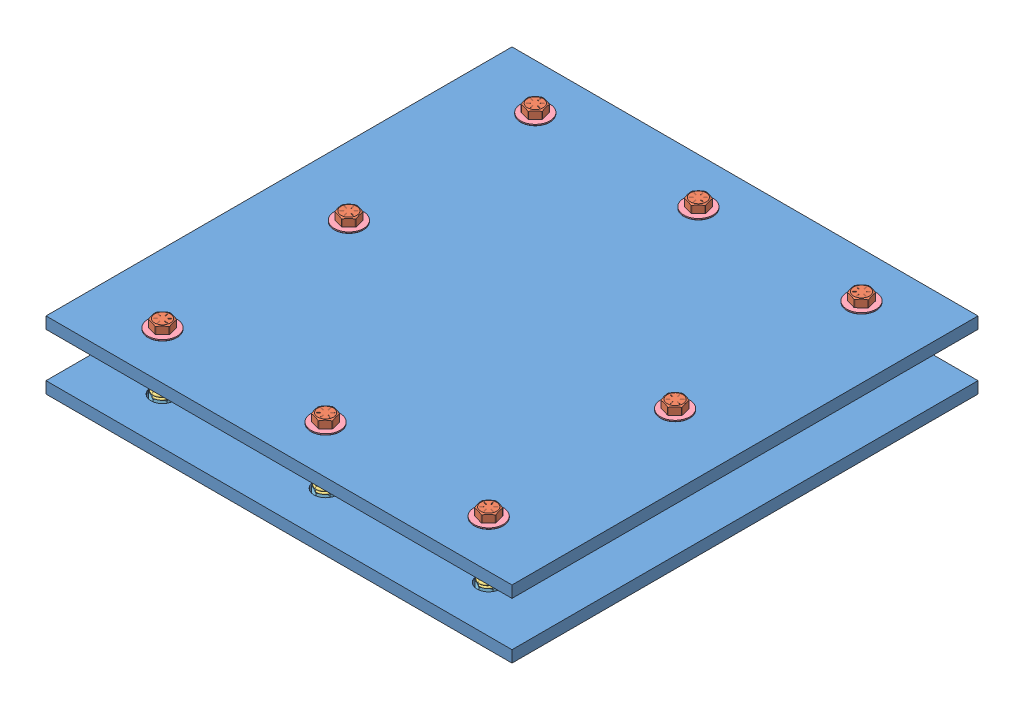
SolidWorks assembly suspension_assem, configuration Default. Lengths in mm.
Overall size (508 85.98 508).
34 component instances, 5 part files, 8 mates.
Components (placement in the parent):
- baseplate-1: baseplate [Default] at (-30.1985 2.5147 9.9128) size (508 12.7 508)
- 92620A724_Zinc Yellow-Chromate Plated Hex Head Screw-1: 92620A724_Zinc Yellow-Chromate Plated Hex Head Screw [92620A724] at (147.6015 16.7895 213.1128) x (0 -1 0) z (-0.270952 0 0.962593) size (85.98 21.7 19.05)
- 9657K31_Compression Spring-1: 9657K31_Compression Spring [9657K31] at (147.6015 12.5847 213.1128) x (-0.104962 0 0.994476) z (0 1 0) size (23.85 23.85 58.72)
- 90107A033_316 Stainless Steel Washer-1: 90107A033_316 Stainless Steel Washer [90107A033] at (147.6015 16.0021 213.1128) x (0.999961 0 0.008869) z (0 -1 0) size (31.75 31.75 1.57)
- 98797A523_Medium-Strength Steel Hex Nuts - Grade 5-1: 98797A523_Medium-Strength Steel Hex Nuts - Grade 5 [98797A523] at (147.6015 -49.9015 213.1128) x (-0.999115 0 0.042064) z (0 -1 0) size (19.05 22 12.65)
- baseplate-2: baseplate [Default] at (-30.1985 -58.6077 9.9128) size (508 12.7 508)
- 98797A523_Medium-Strength Steel Hex Nuts - Grade 5-2: 98797A523_Medium-Strength Steel Hex Nuts - Grade 5 [98797A523] at (147.6015 -49.9015 9.9128) x (-0.999115 0 0.042064) z (0 -1 0) size (19.05 22 12.65)
- 98797A523_Medium-Strength Steel Hex Nuts - Grade 5-3: 98797A523_Medium-Strength Steel Hex Nuts - Grade 5 [98797A523] at (147.6015 -49.9015 -193.2872) x (-0.999115 0 0.042064) z (0 -1 0) size (19.05 22 12.65)
- 98797A523_Medium-Strength Steel Hex Nuts - Grade 5-4: 98797A523_Medium-Strength Steel Hex Nuts - Grade 5 [98797A523] at (-30.1985 -49.9015 213.1128) x (-0.999115 0 0.042064) z (0 -1 0) size (19.05 22 12.65)
- 98797A523_Medium-Strength Steel Hex Nuts - Grade 5-6: 98797A523_Medium-Strength Steel Hex Nuts - Grade 5 [98797A523] at (-30.1985 -49.9015 -193.2872) x (-0.999115 0 0.042064) z (0 -1 0) size (19.05 22 12.65)
- 98797A523_Medium-Strength Steel Hex Nuts - Grade 5-7: 98797A523_Medium-Strength Steel Hex Nuts - Grade 5 [98797A523] at (-207.9985 -49.9015 213.1128) x (-0.999115 0 0.042064) z (0 -1 0) size (19.05 22 12.65)
- 98797A523_Medium-Strength Steel Hex Nuts - Grade 5-8: 98797A523_Medium-Strength Steel Hex Nuts - Grade 5 [98797A523] at (-207.9985 -49.9015 9.9128) x (-0.999115 0 0.042064) z (0 -1 0) size (19.05 22 12.65)
- 98797A523_Medium-Strength Steel Hex Nuts - Grade 5-9: 98797A523_Medium-Strength Steel Hex Nuts - Grade 5 [98797A523] at (-207.9985 -49.9015 -193.2872) x (-0.999115 0 0.042064) z (0 -1 0) size (19.05 22 12.65)
- 9657K31_Compression Spring-2: 9657K31_Compression Spring [9657K31] at (147.6015 12.5847 9.9128) x (-0.104962 0 0.994476) z (0 1 0) size (23.85 23.85 58.72)
- 9657K31_Compression Spring-3: 9657K31_Compression Spring [9657K31] at (147.6015 12.5847 -193.2872) x (-0.104962 0 0.994476) z (0 1 0) size (23.85 23.85 58.72)
- 9657K31_Compression Spring-4: 9657K31_Compression Spring [9657K31] at (-30.1985 12.5847 213.1128) x (-0.104962 0 0.994476) z (0 1 0) size (23.85 23.85 58.72)
- 9657K31_Compression Spring-6: 9657K31_Compression Spring [9657K31] at (-30.1985 12.5847 -193.2872) x (-0.104962 0 0.994476) z (0 1 0) size (23.85 23.85 58.72)
- 9657K31_Compression Spring-7: 9657K31_Compression Spring [9657K31] at (-207.9985 12.5847 213.1128) x (-0.104962 0 0.994476) z (0 1 0) size (23.85 23.85 58.72)
- 9657K31_Compression Spring-8: 9657K31_Compression Spring [9657K31] at (-207.9985 12.5847 9.9128) x (-0.104962 0 0.994476) z (0 1 0) size (23.85 23.85 58.72)
- 9657K31_Compression Spring-9: 9657K31_Compression Spring [9657K31] at (-207.9985 12.5847 -193.2872) x (-0.104962 0 0.994476) z (0 1 0) size (23.85 23.85 58.72)
- 90107A033_316 Stainless Steel Washer-4: 90107A033_316 Stainless Steel Washer [90107A033] at (147.6015 16.0021 9.9128) x (0.999961 0 0.008869) z (0 -1 0) size (31.75 31.75 1.57)
- 90107A033_316 Stainless Steel Washer-5: 90107A033_316 Stainless Steel Washer [90107A033] at (147.6015 16.0021 -193.2872) x (0.999961 0 0.008869) z (0 -1 0) size (31.75 31.75 1.57)
- 90107A033_316 Stainless Steel Washer-6: 90107A033_316 Stainless Steel Washer [90107A033] at (-30.1985 16.0021 213.1128) x (0.999961 0 0.008869) z (0 -1 0) size (31.75 31.75 1.57)
- 90107A033_316 Stainless Steel Washer-8: 90107A033_316 Stainless Steel Washer [90107A033] at (-30.1985 16.0021 -193.2872) x (0.999961 0 0.008869) z (0 -1 0) size (31.75 31.75 1.57)
- 90107A033_316 Stainless Steel Washer-9: 90107A033_316 Stainless Steel Washer [90107A033] at (-207.9985 16.0021 213.1128) x (0.999961 0 0.008869) z (0 -1 0) size (31.75 31.75 1.57)
- 90107A033_316 Stainless Steel Washer-10: 90107A033_316 Stainless Steel Washer [90107A033] at (-207.9985 16.0021 9.9128) x (0.999961 0 0.008869) z (0 -1 0) size (31.75 31.75 1.57)
- 90107A033_316 Stainless Steel Washer-11: 90107A033_316 Stainless Steel Washer [90107A033] at (-207.9985 16.0021 -193.2872) x (0.999961 0 0.008869) z (0 -1 0) size (31.75 31.75 1.57)
- 92620A724_Zinc Yellow-Chromate Plated Hex Head Screw-2: 92620A724_Zinc Yellow-Chromate Plated Hex Head Screw [92620A724] at (147.6015 16.7895 9.9128) x (0 -1 0) z (-0.270952 0 0.962593) size (85.98 21.7 19.05)
- 92620A724_Zinc Yellow-Chromate Plated Hex Head Screw-3: 92620A724_Zinc Yellow-Chromate Plated Hex Head Screw [92620A724] at (147.6015 16.7895 -193.2872) x (0 -1 0) z (-0.270952 0 0.962593) size (85.98 21.7 19.05)
- 92620A724_Zinc Yellow-Chromate Plated Hex Head Screw-4: 92620A724_Zinc Yellow-Chromate Plated Hex Head Screw [92620A724] at (-30.1985 16.7895 213.1128) x (0 -1 0) z (-0.270952 0 0.962593) size (85.98 21.7 19.05)
- 92620A724_Zinc Yellow-Chromate Plated Hex Head Screw-6: 92620A724_Zinc Yellow-Chromate Plated Hex Head Screw [92620A724] at (-30.1985 16.7895 -193.2872) x (0 -1 0) z (-0.270952 0 0.962593) size (85.98 21.7 19.05)
- 92620A724_Zinc Yellow-Chromate Plated Hex Head Screw-7: 92620A724_Zinc Yellow-Chromate Plated Hex Head Screw [92620A724] at (-207.9985 16.7895 213.1128) x (0 -1 0) z (-0.270952 0 0.962593) size (85.98 21.7 19.05)
- 92620A724_Zinc Yellow-Chromate Plated Hex Head Screw-8: 92620A724_Zinc Yellow-Chromate Plated Hex Head Screw [92620A724] at (-207.9985 16.7895 9.9128) x (0 -1 0) z (-0.270952 0 0.962593) size (85.98 21.7 19.05)
- 92620A724_Zinc Yellow-Chromate Plated Hex Head Screw-9: 92620A724_Zinc Yellow-Chromate Plated Hex Head Screw [92620A724] at (-207.9985 16.7895 -193.2872) x (0 -1 0) z (-0.270952 0 0.962593) size (85.98 21.7 19.05)
Mates (geometry in assembly coordinates):
- Concentric1: concentric anti-aligned: circle of baseplate-1; circle of 92620A724_Zinc Yellow-Chromate Plated Hex Head Screw-1
- Concentric2: concentric anti-aligned: circle of 92620A724_Zinc Yellow-Chromate Plated Hex Head Screw-1; circle of 9657K31_Compression Spring-1
- Concentric3: concentric anti-aligned: circle of 92620A724_Zinc Yellow-Chromate Plated Hex Head Screw-1; circle of 90107A033_316 Stainless Steel Washer-1
- Coincident5: coincident anti-aligned: plane of baseplate-1 through (-30.1985 15.2147 9.9128) normal (0 1 0); plane of 90107A033_316 Stainless Steel Washer-1 through (147.6015 15.2147 213.1128) normal (0 -1 0)
- Coincident6: coincident anti-aligned: plane of 92620A724_Zinc Yellow-Chromate Plated Hex Head Screw-1 through (158.1886 16.7895 216.0929) normal (0 -1 0); plane of 90107A033_316 Stainless Steel Washer-1 through (147.6015 16.7895 213.1128) normal (0 1 0)
- Concentric5: concentric aligned: circle of 92620A724_Zinc Yellow-Chromate Plated Hex Head Screw-1; circle of 98797A523_Medium-Strength Steel Hex Nuts - Grade 5-1
- Concentric6: concentric anti-aligned: circle of 92620A724_Zinc Yellow-Chromate Plated Hex Head Screw-1; circle of baseplate-2
- Parallel2: parallel aligned: plane of baseplate-1 through (223.8015 15.2147 263.9128) normal (0 0 1); plane of baseplate-2 through (223.8015 -45.9077 263.9128) normal (0 0 1)
